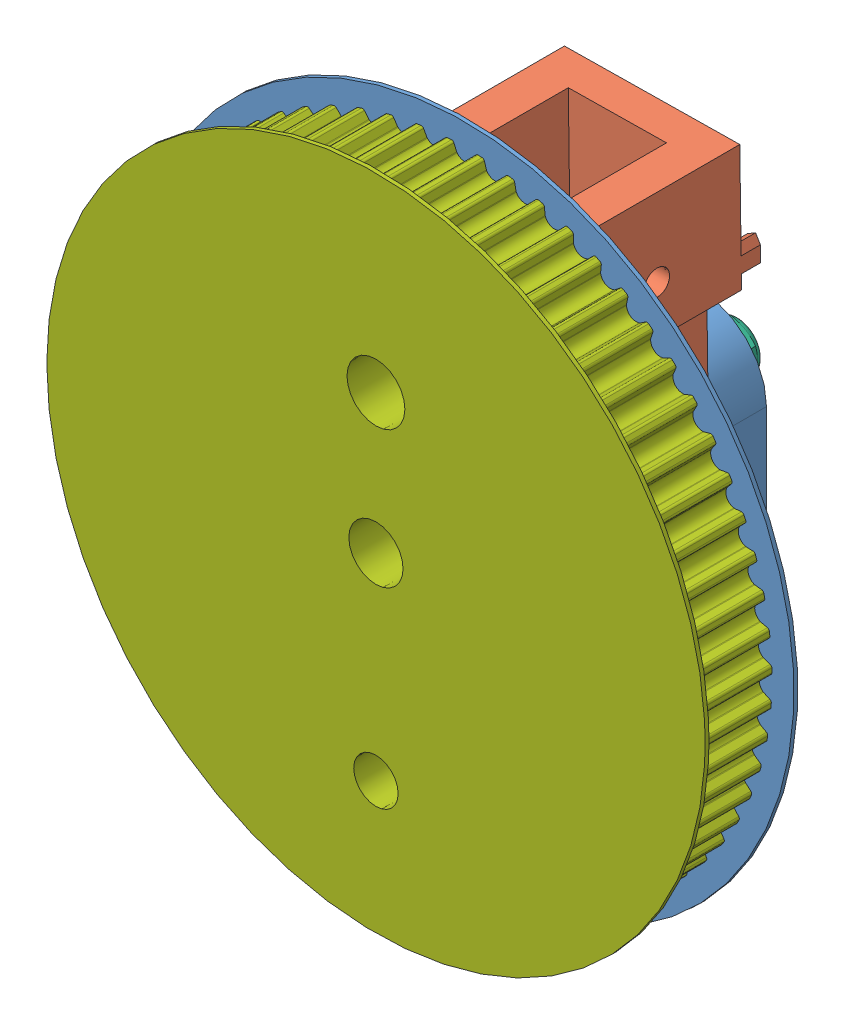
SolidWorks assembly knee_joint, configuration Default. Lengths in mm.
Overall size (170.43 170.43 95.7).
38 component instances, 10 part files, 69 mates.
Components (placement in the parent):
- knee_lower_bracket-1: knee_lower_bracket [Default] at (0 50 0) x (-1 0 0) z (0 0 1) size (170.43 170.43 60.4)
- knee_upper_bracket-1: knee_upper_bracket [Default] at (-0.2197 99.9985 0) x (0.999906 0.013735 0) z (0 0 1) size (45.4 83.67 48.4)
- 5972K91_Ball Bearing-1: 5972K91_Ball Bearing [5972K91] at (0 84.005 21.7) size (22 22 7)
- 5972K91_Ball Bearing-2: 5972K91_Ball Bearing [5972K91] at (0 84.005 -21.7) size (22 22 7)
- 91290A460_Black-Oxide Alloy Steel Socket Head Screw-1: 91290A460_Black-Oxide Alloy Steel Socket Head Screw [91290A460] at (0 84.005 -5.8) size (13 13 78.54)
- knee_spacer-1: knee_spacer [Default] at (0 84.005 -29.45) size (13 13 8.5)
- 93625A114_18-8 Stainless Steel Nylon-Insert Locknut-1: 93625A114_18-8 Stainless Steel Nylon-Insert Locknut [93625A114] at (0 84.005 -38.45) x (1 0 0) z (0 1 0) size (13 9.54 15.01)
- knee_pulley-1: knee_pulley [Default] at (0 84.005 49.7) x (-1 0 0) z (0 0 -1) size (170.43 170.43 23)
- 94459A140_Brass Heat-Set Inserts for Plastic-1: 94459A140_Brass Heat-Set Inserts for Plastic [94459A140] at (45.9619 129.9669 33.4) x (1 0 0) z (0 1 0) size (4.77 6.11 4.77)
- 94459A140_Brass Heat-Set Inserts for Plastic-3: 94459A140_Brass Heat-Set Inserts for Plastic [94459A140] at (62.7852 67.1818 33.4) x (1 0 0) z (0 1 0) size (4.77 6.11 4.77)
- 94459A140_Brass Heat-Set Inserts for Plastic-4: 94459A140_Brass Heat-Set Inserts for Plastic [94459A140] at (35 24.005 33.4) x (1 0 0) z (0 1 0) size (4.77 6.11 4.77)
- 94459A140_Brass Heat-Set Inserts for Plastic-5: 94459A140_Brass Heat-Set Inserts for Plastic [94459A140] at (25 19.005 33.4) x (1 0 0) z (0 1 0) size (4.77 6.11 4.77)
- 94459A140_Brass Heat-Set Inserts for Plastic-7: 94459A140_Brass Heat-Set Inserts for Plastic [94459A140] at (22.75 84.005 33.4) x (1 0 0) z (0 1 0) size (4.77 6.11 4.77)
- 94459A140_Brass Heat-Set Inserts for Plastic-14: 94459A140_Brass Heat-Set Inserts for Plastic [94459A140] at (22.75 59.005 33.4) x (1 0 0) z (0 1 0) size (4.77 6.11 4.77)
- 94459A140_Brass Heat-Set Inserts for Plastic-15: 94459A140_Brass Heat-Set Inserts for Plastic [94459A140] at (0 106.755 33.4) x (1 0 0) z (0 1 0) size (4.77 6.11 4.77)
- 94459A140_Brass Heat-Set Inserts for Plastic-17: 94459A140_Brass Heat-Set Inserts for Plastic [94459A140] at (40.0705 49.005 33.4) x (1 0 0) z (0 1 0) size (4.77 6.11 4.77)
- 92095A472_Button Head Hex Drive Screw-1: 92095A472_Button Head Hex Drive Screw [92095A472] at (45.9619 129.9669 25.05) x (-1 0 0) z (0 0 -1) size (5.7 5.7 20.01)
- 92095A472_Button Head Hex Drive Screw-2: 92095A472_Button Head Hex Drive Screw [92095A472] at (62.7852 67.1818 25.05) x (-1 0 0) z (0 0 -1) size (5.7 5.7 20.01)
- 92095A472_Button Head Hex Drive Screw-3: 92095A472_Button Head Hex Drive Screw [92095A472] at (22.75 84.005 23.05) x (-1 0 0) z (0 0 -1) size (5.7 5.7 20.01)
- 92095A472_Button Head Hex Drive Screw-7: 92095A472_Button Head Hex Drive Screw [92095A472] at (22.75 59.005 23.05) x (-1 0 0) z (0 0 -1) size (5.7 5.7 20.01)
- 92095A472_Button Head Hex Drive Screw-8: 92095A472_Button Head Hex Drive Screw [92095A472] at (0 106.755 23.05) x (-1 0 0) z (0 0 -1) size (5.7 5.7 20.01)
- 92095A473_Button Head Hex Drive Screw-1: 92095A473_Button Head Hex Drive Screw [92095A473] at (25 19.005 16.05) x (-1 0 0) z (0 0 -1) size (5.7 5.7 24.04)
- 92095A473_Button Head Hex Drive Screw-2: 92095A473_Button Head Hex Drive Screw [92095A473] at (35 24.005 16.05) x (-1 0 0) z (0 0 -1) size (5.7 5.7 24.04)
- 94459A140_Brass Heat-Set Inserts for Plastic-9: 94459A140_Brass Heat-Set Inserts for Plastic [94459A140] at (-45.9619 129.9669 27.6889) x (-1 0 0) z (0 1 0) size (4.77 6.11 4.77)
- 92095A473_Button Head Hex Drive Screw-3: 92095A473_Button Head Hex Drive Screw [92095A473] at (-35 24.005 16.05) x (1 0 0) z (0 0 -1) size (5.7 5.7 24.04)
- 92095A473_Button Head Hex Drive Screw-4: 92095A473_Button Head Hex Drive Screw [92095A473] at (-25 19.005 16.05) x (1 0 0) z (0 0 -1) size (5.7 5.7 24.04)
- 92095A472_Button Head Hex Drive Screw-4: 92095A472_Button Head Hex Drive Screw [92095A472] at (-22.75 84.005 23.05) x (1 0 0) z (0 0 -1) size (5.7 5.7 20.01)
- 92095A472_Button Head Hex Drive Screw-5: 92095A472_Button Head Hex Drive Screw [92095A472] at (-62.7852 67.1818 25.05) x (1 0 0) z (0 0 -1) size (5.7 5.7 20.01)
- 92095A472_Button Head Hex Drive Screw-6: 92095A472_Button Head Hex Drive Screw [92095A472] at (-45.9619 129.9669 25.05) x (1 0 0) z (0 0 -1) size (5.7 5.7 20.01)
- 94459A140_Brass Heat-Set Inserts for Plastic-10: 94459A140_Brass Heat-Set Inserts for Plastic [94459A140] at (-22.75 84.005 27.6889) x (-1 0 0) z (0 1 0) size (4.77 6.11 4.77)
- 94459A140_Brass Heat-Set Inserts for Plastic-11: 94459A140_Brass Heat-Set Inserts for Plastic [94459A140] at (-25 19.005 27.6889) x (-1 0 0) z (0 1 0) size (4.77 6.11 4.77)
- 94459A140_Brass Heat-Set Inserts for Plastic-12: 94459A140_Brass Heat-Set Inserts for Plastic [94459A140] at (-35 24.005 27.6889) x (-1 0 0) z (0 1 0) size (4.77 6.11 4.77)
- 94459A140_Brass Heat-Set Inserts for Plastic-13: 94459A140_Brass Heat-Set Inserts for Plastic [94459A140] at (-62.7852 67.1818 27.6889) x (-1 0 0) z (0 1 0) size (4.77 6.11 4.77)
- 94459A140_Brass Heat-Set Inserts for Plastic-16: 94459A140_Brass Heat-Set Inserts for Plastic [94459A140] at (-22.75 59.005 27.6889) x (-1 0 0) z (0 1 0) size (4.77 6.11 4.77)
- 92095A472_Button Head Hex Drive Screw-9: 92095A472_Button Head Hex Drive Screw [92095A472] at (-22.75 59.005 23.05) x (1 0 0) z (0 0 -1) size (5.7 5.7 20.01)
- 92095A472_Button Head Hex Drive Screw-10: 92095A472_Button Head Hex Drive Screw [92095A472] at (40.0705 49.005 23.05) x (-1 0 0) z (0 0 -1) size (5.7 5.7 20.01)
- 92095A472_Button Head Hex Drive Screw-11: 92095A472_Button Head Hex Drive Screw [92095A472] at (-40.0705 49.005 23.05) x (1 0 0) z (0 0 -1) size (5.7 5.7 20.01)
- 94459A140_Brass Heat-Set Inserts for Plastic-18: 94459A140_Brass Heat-Set Inserts for Plastic [94459A140] at (-40.0705 49.005 27.6889) x (-1 0 0) z (0 1 0) size (4.77 6.11 4.77)
Mates (geometry in assembly coordinates):
- Concentric1: concentric anti-aligned: cylinder of knee_upper_bracket-1 through (0 84.005 60.2872) axis (0 0 -1) radius 4.025; cylinder of 5972K91_Ball Bearing-1 through (0 84.005 25.2) axis (0 0 1) radius 4
- Coincident1: coincident anti-aligned: plane of knee_upper_bracket-1 through (-0.2197 99.9985 18.2) normal (0 0 1); plane of 5972K91_Ball Bearing-1 through (0 88.355 18.2) normal (0 0 -1)
- Concentric2: concentric anti-aligned: cylinder of knee_lower_bracket-1 through (0 84.005 32.7) axis (0 0 -1) radius 7.025; cylinder of 5972K91_Ball Bearing-1 through (0 84.005 25.2) axis (0 0 1) radius 11
- Parallel1: parallel aligned: plane of 5972K91_Ball Bearing-1 through (0 84.005 21.7) normal (1 0 0)
- Concentric4: concentric anti-aligned: cylinder of knee_upper_bracket-1 through (0 84.005 60.2872) axis (0 0 -1) radius 4.025; cylinder of 5972K91_Ball Bearing-2 through (0 84.005 -18.2) axis (0 0 1) radius 4
- Coincident7: coincident anti-aligned: plane of knee_upper_bracket-1 through (-0.2197 99.9985 -18.2) normal (0 0 -1); plane of 5972K91_Ball Bearing-2 through (0 90.8457 -18.2) normal (0 0 1)
- Parallel2: parallel aligned: plane of 5972K91_Ball Bearing-2 through (0 84.005 -21.7) normal (1 0 0)
- Concentric5: concentric anti-aligned: cylinder of 5972K91_Ball Bearing-1 through (0 84.005 25.2) axis (0 0 1) radius 4; cylinder of 90128A281_Zinc-Plated Alloy Steel Socket Head Screw-1 through (0 81 79.1195) axis (0 0 -1) radius 4.127
- Concentric6: concentric anti-aligned: cylinder of 5972K91_Ball Bearing-1 through (0 84.005 25.2) axis (0 0 1) radius 4; cylinder of 91290A460_Black-Oxide Alloy Steel Socket Head Screw-1 through (0 84.005 -44.8) axis (0 0 -1) radius 4
- Coincident13: coincident anti-aligned: plane of 5972K91_Ball Bearing-1 through (0 90.8457 25.2) normal (0 0 1); plane of 91290A460_Black-Oxide Alloy Steel Socket Head Screw-1 through (0 90.105 25.2) normal (0 0 -1)
- Parallel3: parallel aligned: plane of 91290A460_Black-Oxide Alloy Steel Socket Head Screw-1 through (0 84.005 -5.8) normal (1 0 0)
- Coincident14: coincident anti-aligned: plane of 5972K91_Ball Bearing-2 through (0 88.355 -25.2) normal (0 0 -1); plane of knee_spacer-1 through (0 84.005 -25.2) normal (0 0 1)
- Concentric7: concentric aligned: cylinder of 91290A460_Black-Oxide Alloy Steel Socket Head Screw-1 through (0 84.005 -44.8) axis (0 0 -1) radius 4; cylinder of knee_spacer-1 through (0 84.005 -25.2) axis (0 0 -1) radius 4.025
- Parallel4: parallel aligned: plane of knee_spacer-1 through (0 84.005 -29.45) normal (1 0 0)
- Coincident16: coincident anti-aligned: plane of knee_spacer-1 through (0 84.005 -33.7) normal (0 0 -1); plane of 93625A114_18-8 Stainless Steel Nylon-Insert Locknut-1 through (0 84.005 -33.7) normal (0 0 1)
- Concentric8: concentric anti-aligned: cylinder of 91290A460_Black-Oxide Alloy Steel Socket Head Screw-1 through (0 84.005 -44.8) axis (0 0 -1) radius 4; cylinder of 93625A114_18-8 Stainless Steel Nylon-Insert Locknut-1 through (0 84.005 -38.45) axis (0 0 1) radius 3.2188
- Parallel5: parallel aligned: plane of 93625A114_18-8 Stainless Steel Nylon-Insert Locknut-1 through (0 84.005 -38.45) normal (1 0 0)
- Width1: width anti-aligned: plane of knee_lower_bracket-1 through (0 84.005 -25.205) normal (0 0 1); plane of 5972K91_Ball Bearing-2 through (0 84.005 25.205) normal (0 0 -1); plane of knee_lower_bracket-1 through (0 94.655 -25.2) normal (0 0 -1); plane of 5972K91_Ball Bearing-1 through (0 94.655 25.2) normal (0 0 1)
- Coincident17: coincident anti-aligned: plane of knee_lower_bracket-1 through (0 50 27.7) normal (0 0 1); plane of knee_pulley-1 through (0 84.005 27.7) normal (0 0 -1)
- Concentric9: concentric anti-aligned: cylinder of knee_lower_bracket-1 through (45.9619 129.9669 -32.7) axis (0 0 1) radius 1.7; cylinder of knee_pulley-1 through (45.9619 129.9669 45.7) axis (0 0 -1) radius 1.985
- Concentric10: concentric anti-aligned: cylinder of knee_lower_bracket-1 through (-45.9619 129.9669 -32.7) axis (0 0 1) radius 1.7; cylinder of knee_pulley-1 through (-45.9619 129.9669 45.7) axis (0 0 -1) radius 1.985
- Coincident18: coincident anti-aligned: plane of knee_lower_bracket-1 through (0 50 26.7) normal (0 0 -1); plane of 92095A472_Button Head Hex Drive Screw-1 through (43.1119 129.9669 26.7) normal (0 0 1)
- Concentric11: concentric anti-aligned: cylinder of knee_lower_bracket-1 through (45.9619 129.9669 -32.7) axis (0 0 1) radius 1.7; cylinder of 92095A472_Button Head Hex Drive Screw-1 through (45.9619 129.9669 25.05) axis (0 0 -1) radius 2.85
- Coincident19: coincident anti-aligned: plane of knee_lower_bracket-1 through (0 50 26.7) normal (0 0 -1); plane of 92095A472_Button Head Hex Drive Screw-2 through (59.9352 67.1818 26.7) normal (0 0 1)
- Concentric12: concentric anti-aligned: cylinder of knee_lower_bracket-1 through (62.7852 67.1818 -32.7) axis (0 0 1) radius 1.7; cylinder of 92095A472_Button Head Hex Drive Screw-2 through (62.7852 67.1818 25.05) axis (0 0 -1) radius 2.85
- Concentric13: concentric aligned: cylinder of knee_lower_bracket-1 through (25 19.005 27.7) axis (0 0 -1) radius 1.7; cylinder of 92095A473_Button Head Hex Drive Screw-1 through (25 19.005 16.05) axis (0 0 -1) radius 2.85
- Coincident20: coincident anti-aligned: plane of knee_lower_bracket-1 through (0 50 17.7) normal (0 0 -1); plane of 92095A473_Button Head Hex Drive Screw-1 through (22.15 19.005 17.7) normal (0 0 1)
- Concentric14: concentric aligned: cylinder of knee_lower_bracket-1 through (35 24.005 27.7) axis (0 0 -1) radius 1.7; cylinder of 92095A473_Button Head Hex Drive Screw-2 through (35 24.005 16.05) axis (0 0 -1) radius 2.85
- Coincident21: coincident anti-aligned: plane of knee_lower_bracket-1 through (0 50 17.7) normal (0 0 -1); plane of 92095A473_Button Head Hex Drive Screw-2 through (32.15 24.005 17.7) normal (0 0 1)
- Concentric15: concentric anti-aligned: cylinder of knee_lower_bracket-1 through (22.75 84.005 24.7) axis (0 0 1) radius 1.7; cylinder of 92095A472_Button Head Hex Drive Screw-3 through (22.75 84.005 23.05) axis (0 0 -1) radius 2.85
- Coincident22: coincident anti-aligned: plane of knee_lower_bracket-1 through (0 50 24.7) normal (0 0 -1); plane of 92095A472_Button Head Hex Drive Screw-3 through (19.9 84.005 24.7) normal (0 0 1)
- Parallel6: parallel aligned: plane of knee_lower_bracket-1 through (0 50 0) normal (-1 0 0); plane of 92095A472_Button Head Hex Drive Screw-1 through (45.9619 129.9669 25.05) normal (-1 0 0)
- Parallel7: parallel aligned: plane of knee_lower_bracket-1 through (0 50 0) normal (-1 0 0); plane of 92095A472_Button Head Hex Drive Screw-2 through (62.7852 67.1818 25.05) normal (-1 0 0)
- Parallel8: parallel aligned: plane of knee_lower_bracket-1 through (0 50 0) normal (-1 0 0); plane of 92095A473_Button Head Hex Drive Screw-1 through (25 19.005 16.05) normal (-1 0 0)
- Parallel9: parallel aligned: plane of knee_lower_bracket-1 through (0 50 0) normal (-1 0 0); plane of 92095A473_Button Head Hex Drive Screw-2 through (35 24.005 16.05) normal (-1 0 0)
- Parallel10: parallel aligned: plane of knee_lower_bracket-1 through (0 50 0) normal (-1 0 0); plane of 92095A472_Button Head Hex Drive Screw-3 through (22.75 84.005 23.05) normal (-1 0 0)
- Concentric16: concentric anti-aligned: cylinder of knee_pulley-1 through (45.9619 129.9669 45.7) axis (0 0 -1) radius 1.985; cylinder of 94459A140_Brass Heat-Set Inserts for Plastic-1 through (45.9619 129.9669 33.4) axis (0 0 1) radius 1.95
- Coincident23: coincident aligned: plane of knee_pulley-1 through (0 84.005 27.7) normal (0 0 -1); plane of 94459A140_Brass Heat-Set Inserts for Plastic-1 through (48.3119 129.9669 27.7) normal (0 0 -1)
- Parallel11: parallel anti-aligned: plane of knee_pulley-1 through (0 84.005 49.7) normal (-1 0 0); plane of 94459A140_Brass Heat-Set Inserts for Plastic-1 through (45.9619 129.9669 33.4) normal (1 0 0)
- Coincident24: coincident aligned: plane of knee_pulley-1 through (0 84.005 27.7) normal (0 0 -1); plane of 94459A140_Brass Heat-Set Inserts for Plastic-3 through (65.1352 67.1818 27.7) normal (0 0 -1)
- Parallel12: parallel anti-aligned: plane of knee_pulley-1 through (0 84.005 49.7) normal (-1 0 0); plane of 94459A140_Brass Heat-Set Inserts for Plastic-3 through (62.7852 67.1818 33.4) normal (1 0 0)
- Concentric17: concentric anti-aligned: cylinder of knee_pulley-1 through (62.7852 67.1818 45.7) axis (0 0 -1) radius 1.985; cylinder of 94459A140_Brass Heat-Set Inserts for Plastic-3 through (62.7852 67.1818 33.4) axis (0 0 1) radius 1.95
- Coincident25: coincident aligned: plane of knee_pulley-1 through (0 84.005 27.7) normal (0 0 -1); plane of 94459A140_Brass Heat-Set Inserts for Plastic-4 through (37.35 24.005 27.7) normal (0 0 -1)
- Parallel13: parallel anti-aligned: plane of knee_pulley-1 through (0 84.005 49.7) normal (-1 0 0); plane of 94459A140_Brass Heat-Set Inserts for Plastic-4 through (35 24.005 33.4) normal (1 0 0)
- Concentric18: concentric anti-aligned: cylinder of knee_pulley-1 through (35 24.005 45.7) axis (0 0 -1) radius 1.985; cylinder of 94459A140_Brass Heat-Set Inserts for Plastic-4 through (35 24.005 33.4) axis (0 0 1) radius 1.95
- Coincident26: coincident aligned: plane of knee_pulley-1 through (0 84.005 27.7) normal (0 0 -1); plane of 94459A140_Brass Heat-Set Inserts for Plastic-5 through (27.35 19.005 27.7) normal (0 0 -1)
- Parallel14: parallel anti-aligned: plane of knee_pulley-1 through (0 84.005 49.7) normal (-1 0 0); plane of 94459A140_Brass Heat-Set Inserts for Plastic-5 through (25 19.005 33.4) normal (1 0 0)
- Concentric19: concentric anti-aligned: cylinder of knee_pulley-1 through (25 19.005 45.7) axis (0 0 -1) radius 1.985; cylinder of 94459A140_Brass Heat-Set Inserts for Plastic-5 through (25 19.005 33.4) axis (0 0 1) radius 1.95
- Parallel16: parallel anti-aligned: plane of knee_pulley-1 through (0 84.005 49.7) normal (-1 0 0); plane of 94459A140_Brass Heat-Set Inserts for Plastic-7 through (22.75 84.005 33.4) normal (1 0 0)
- Coincident28: coincident aligned: plane of knee_pulley-1 through (0 84.005 27.7) normal (0 0 -1); plane of 94459A140_Brass Heat-Set Inserts for Plastic-7 through (25.1 84.005 27.7) normal (0 0 -1)
- Concentric21: concentric anti-aligned: cylinder of knee_pulley-1 through (22.75 84.005 45.7) axis (0 0 -1) radius 1.985; cylinder of 94459A140_Brass Heat-Set Inserts for Plastic-7 through (22.75 84.005 33.4) axis (0 0 1) radius 1.95
- Concentric22: concentric anti-aligned: cylinder of knee_pulley-1 through (22.75 59.005 45.7) axis (0 0 -1) radius 1.985; cylinder of 94459A140_Brass Heat-Set Inserts for Plastic-14 through (22.75 59.005 33.4) axis (0 0 1) radius 1.95
- Coincident29: coincident aligned: plane of knee_pulley-1 through (0 84.005 27.7) normal (0 0 -1); plane of 94459A140_Brass Heat-Set Inserts for Plastic-14 through (25.1 59.005 27.7) normal (0 0 -1)
- Parallel17: parallel anti-aligned: plane of knee_pulley-1 through (0 84.005 49.7) normal (-1 0 0); plane of 94459A140_Brass Heat-Set Inserts for Plastic-14 through (22.75 59.005 33.4) normal (1 0 0)
- Concentric23: concentric anti-aligned: cylinder of knee_pulley-1 through (0 106.755 45.7) axis (0 0 -1) radius 1.985; cylinder of 94459A140_Brass Heat-Set Inserts for Plastic-15 through (0 106.755 33.4) axis (0 0 1) radius 1.95
- Coincident30: coincident aligned: plane of knee_pulley-1 through (0 84.005 27.7) normal (0 0 -1); plane of 94459A140_Brass Heat-Set Inserts for Plastic-15 through (2.35 106.755 27.7) normal (0 0 -1)
- Parallel18: parallel anti-aligned: plane of knee_pulley-1 through (0 84.005 49.7) normal (-1 0 0); plane of 94459A140_Brass Heat-Set Inserts for Plastic-15 through (0 106.755 33.4) normal (1 0 0)
- Concentric24: concentric anti-aligned: cylinder of knee_lower_bracket-1 through (22.75 59.005 24.7) axis (0 0 1) radius 1.7; cylinder of 92095A472_Button Head Hex Drive Screw-7 through (22.75 59.005 23.05) axis (0 0 -1) radius 2.85
- Coincident31: coincident anti-aligned: plane of knee_lower_bracket-1 through (0 50 24.7) normal (0 0 -1); plane of 92095A472_Button Head Hex Drive Screw-7 through (19.9 59.005 24.7) normal (0 0 1)
- Parallel19: parallel aligned: plane of knee_lower_bracket-1 through (0 50 0) normal (-1 0 0); plane of 92095A472_Button Head Hex Drive Screw-7 through (22.75 59.005 23.05) normal (-1 0 0)
- Coincident32: coincident anti-aligned: plane of knee_lower_bracket-1 through (0 50 24.7) normal (0 0 -1); plane of 92095A472_Button Head Hex Drive Screw-8 through (-2.85 106.755 24.7) normal (0 0 1)
- Concentric25: concentric anti-aligned: cylinder of knee_lower_bracket-1 through (0 106.755 24.7) axis (0 0 1) radius 1.7; cylinder of 92095A472_Button Head Hex Drive Screw-8 through (0 106.755 23.05) axis (0 0 -1) radius 2.85
- Parallel20: parallel aligned: plane of knee_lower_bracket-1 through (0 50 0) normal (-1 0 0); plane of 92095A472_Button Head Hex Drive Screw-8 through (0 106.755 23.05) normal (-1 0 0)
- Concentric26: concentric anti-aligned: cylinder of knee_pulley-1 through (40.0705 49.005 45.7) axis (0 0 -1) radius 1.985; cylinder of 94459A140_Brass Heat-Set Inserts for Plastic-17 through (40.0705 49.005 33.4) axis (0 0 1) radius 1.95
- Coincident33: coincident aligned: plane of knee_pulley-1 through (0 84.005 27.7) normal (0 0 -1); plane of 94459A140_Brass Heat-Set Inserts for Plastic-17 through (42.4205 49.005 27.7) normal (0 0 -1)
- Parallel21: parallel anti-aligned: plane of knee_pulley-1 through (0 84.005 49.7) normal (-1 0 0); plane of 94459A140_Brass Heat-Set Inserts for Plastic-17 through (40.0705 49.005 33.4) normal (1 0 0)
- Concentric27: concentric anti-aligned: cylinder of knee_lower_bracket-1 through (40.0705 49.005 24.7) axis (0 0 1) radius 1.7; cylinder of 92095A472_Button Head Hex Drive Screw-10 through (40.0705 49.005 23.05) axis (0 0 -1) radius 2.85
- Coincident34: coincident anti-aligned: plane of knee_lower_bracket-1 through (0 50 24.7) normal (0 0 -1); plane of 92095A472_Button Head Hex Drive Screw-10 through (37.2205 49.005 24.7) normal (0 0 1)
- Parallel22: parallel aligned: plane of knee_lower_bracket-1 through (0 50 0) normal (-1 0 0); plane of 92095A472_Button Head Hex Drive Screw-10 through (40.0705 49.005 23.05) normal (-1 0 0)
